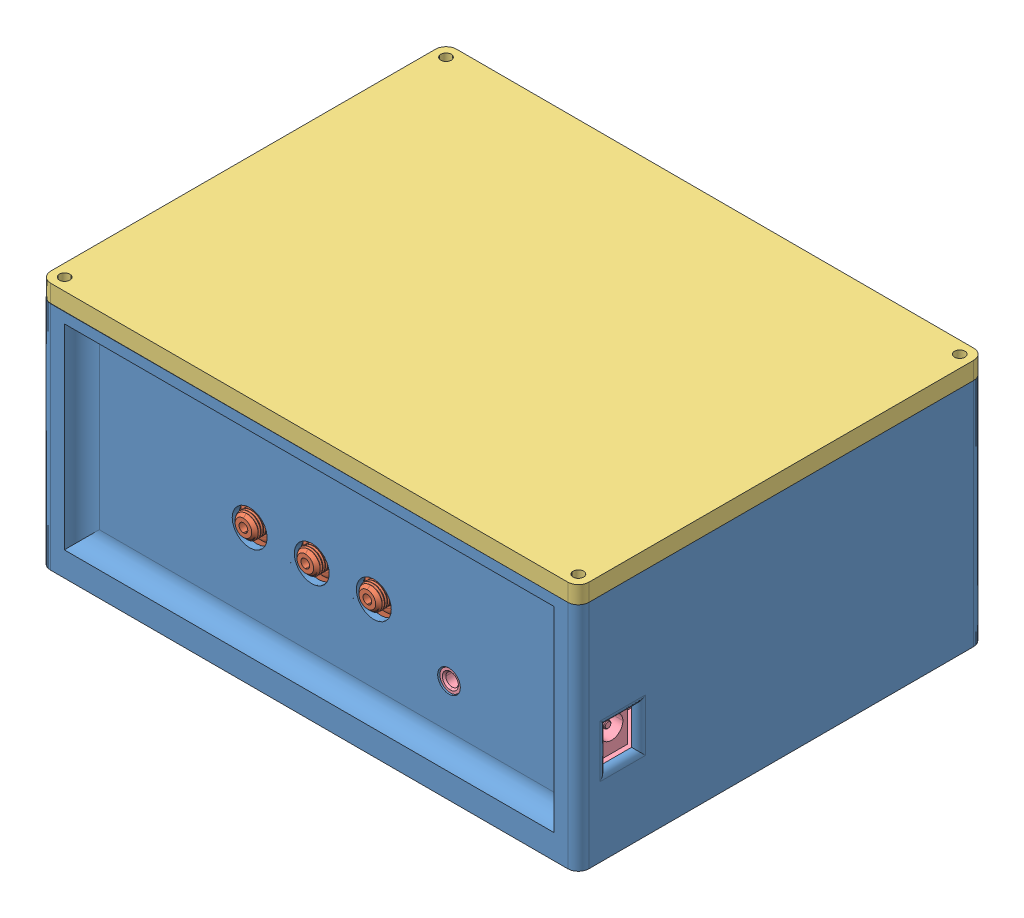
SolidWorks assembly enclosure final, configuration Default. Lengths in mm.
Overall size (154.67 71 116.1).
4 component instances, 4 part files, 6 mates.
Components (placement in the parent):
- volume expander-1: volume expander [Default] at (156.348 150.7416 296.6756) size (154 66 116)
- AnalogProjects.step-2: AnalogProjects.step [Default] at (251.122 172.6512 168.6936) x (-1 0 0) z (0 1 0) size (102.6 105.34 33.98)
- volume expander top-2: volume expander top [Default] at (156.3818 221.7416 296.6301) x (1 0 0.00062) z (0.00062 0 -1) size (154 5 116)
- Power_Pcb.step-2: Power_Pcb.step [Default] at (173.817 172.5535 357.7086) x (1 0 0) z (0 1 0) size (47.5 101.64 33.98)
Mates (geometry in assembly coordinates):
- Coincident2: coincident anti-aligned: plane of volume expander-1 through (81.348 152.7416 347.6756) normal (0 0 -1); plane of AnalogProjects.step-2 through (181.348 172.2398 347.6756) normal (0 0 1)
- Coincident3: coincident anti-aligned: plane of volume expander-1 through (81.348 152.7416 245.6756) normal (1 0 0); plane of AnalogProjects.step-2 through (81.348 172.2398 347.6756) normal (-1 0 0)
- Coincident11: coincident anti-aligned: plane of volume expander-1 through (156.348 216.7416 296.6756) normal (0 1 0); plane of volume expander top-2 through (156.3818 216.7416 296.6301) normal (0 -1 0)
- Concentric1: concentric aligned: cylinder of volume expander-1 through (206.348 160.7416 267.6756) axis (0 1 0) radius 2.1; cylinder of Power_Pcb.step-2 through (206.348 163.3335 267.6756) axis (0 1 0) radius 1.5
- Concentric2: concentric aligned: cylinder of volume expander-1 through (223.348 160.7416 293.6756) axis (0 1 0) radius 2.1; cylinder of Power_Pcb.step-2 through (223.348 163.3335 293.6756) axis (0 1 0) radius 1.5
- Concentric3: concentric anti-aligned: cylinder of volume expander-1 through (229.848 206.7416 351.1756) axis (0 1 0) radius 2.1; cylinder of volume expander top-2 through (229.848 221.7416 351.1756) axis (0 -1 0) radius 1.5
